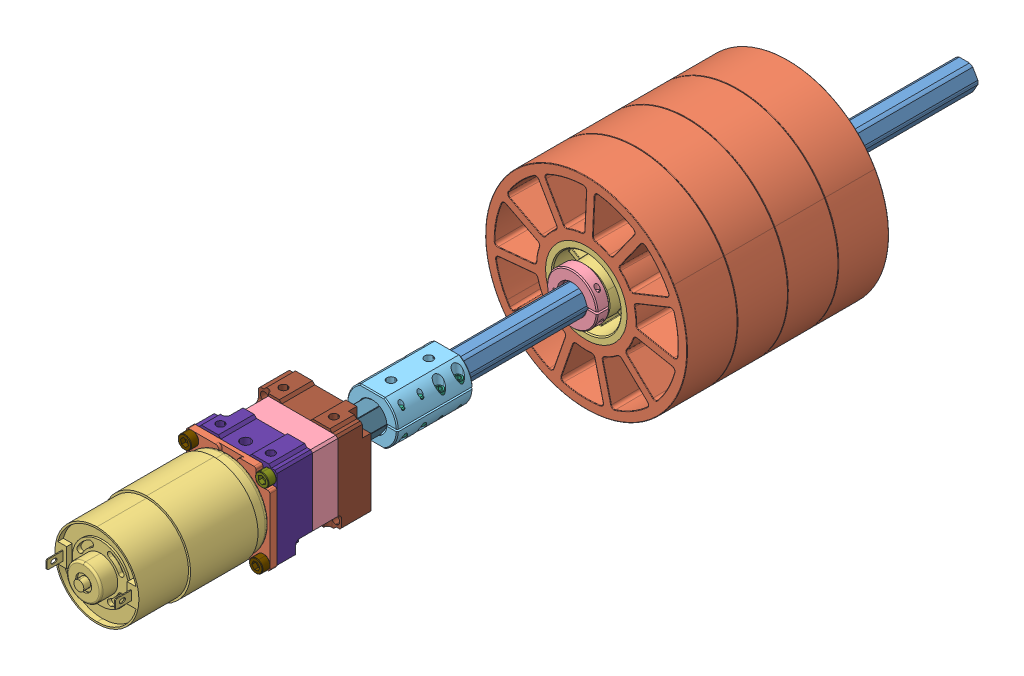
SolidWorks assembly Assem_Launch_Component(wheels,hexshaft,motor,etc.)-SP, configuration Default. Lengths in mm.
Overall size (138.79 138.79 446).
59 component instances, 25 part files, 14 mates.
Components (placement in the parent):
- ThunderHex(.5 11inch)-SP-1: ThunderHex(.5 11inch)-SP [Default] at origin size (13.74 12.75 279.4)
- CompliantWheel(4inch 500)SP-1: CompliantWheel(4inch 500)SP [Default] at (15.9875 4.7838 44.7916) x (0.866025 0.5 0) z (0 0 1) size (101.6 101.6 25.4)
  - CompliantWheel(4inch 500)SP.STEP-1: CompliantWheel(4inch 500)SP.STEP [Default] at origin size (101.6 101.6 25.4)
    - 4IN Compliant Wheel FINAL Overmold.STEP-1: 4IN Compliant Wheel FINAL Overmold.STEP [Default] at (-16.2374 3.8509 18.652) size (101.6 101.6 25.4)
    - 2in Wheel Intergrated 0500 HEX Hub.STEP-1: 2in Wheel Intergrated 0500 HEX Hub.STEP [Default] at (-16.2374 3.8509 5.952) x (-1 0 0) z (0 0 -1) size (41.91 41.91 25.4)
- CompliantWheel(4inch 500)SP.STEP-1: CompliantWheel(4inch 500)SP.STEP [Default] at (15.9875 4.7838 70.1916) x (0.866025 0.5 0) z (0 0 1) size (101.6 101.6 25.4)
  - 4IN Compliant Wheel FINAL Overmold.STEP-1: 4IN Compliant Wheel FINAL Overmold.STEP [Default] at (-16.2374 3.8509 18.652) size (101.6 101.6 25.4)
  - 2in Wheel Intergrated 0500 HEX Hub.STEP-1: 2in Wheel Intergrated 0500 HEX Hub.STEP [Default] at (-16.2374 3.8509 5.952) x (-1 0 0) z (0 0 -1) size (41.91 41.91 25.4)
- CompliantWheel(4inch 500)SP.STEP-3: CompliantWheel(4inch 500)SP.STEP [Default] at (15.9875 4.7838 95.5916) x (0.866025 0.5 0) z (0 0 1) size (101.6 101.6 25.4)
  - 4IN Compliant Wheel FINAL Overmold.STEP-1: 4IN Compliant Wheel FINAL Overmold.STEP [Default] at (-16.2374 3.8509 18.652) size (101.6 101.6 25.4)
  - 2in Wheel Intergrated 0500 HEX Hub.STEP-1: 2in Wheel Intergrated 0500 HEX Hub.STEP [Default] at (-16.2374 3.8509 5.952) x (-1 0 0) z (0 0 -1) size (41.91 41.91 25.4)
- CompliantWheel(4inch 500)SP.STEP-4: CompliantWheel(4inch 500)SP.STEP [Default] at (15.9875 4.7838 120.9916) x (0.866025 0.5 0) z (0 0 1) size (101.6 101.6 25.4)
  - 4IN Compliant Wheel FINAL Overmold.STEP-1: 4IN Compliant Wheel FINAL Overmold.STEP [Default] at (-16.2374 3.8509 18.652) size (101.6 101.6 25.4)
  - 2in Wheel Intergrated 0500 HEX Hub.STEP-1: 2in Wheel Intergrated 0500 HEX Hub.STEP [Default] at (-16.2374 3.8509 5.952) x (-1 0 0) z (0 0 -1) size (41.91 41.91 25.4)
- ClampingShaftCollar(.5 in)SP-1: ClampingShaftCollar(.5 in)SP [Default] at (0 -0.2032 34.8687) size (25.39 25.4 6.35)
- ClampingShaftCollar(.5 in)SP-2: ClampingShaftCollar(.5 in)SP [Default] at (-0.8969 -0.0987 142.8187) size (25.39 25.4 6.35)
- Hex_Shaft_Coupler(.5)-SP-1: Hex_Shaft_Coupler(.5)-SP [Default] at (0.04 0 228.4754) size (25.76 22.32 38.1)
  - Hex_Shaft_Coupler(.5)-SP.STEP-1: Hex_Shaft_Coupler(.5)-SP.STEP [Default] at origin size (25.76 22.32 38.1)
    - 217-4008-001 Rev1.STEP-1: 217-4008-001 Rev1.STEP [Default] at origin size (25.38 10.66 38.1)
    - 217-4008-001 Rev1.STEP-2: 217-4008-001 Rev1.STEP [Default] x (1 0 0) z (0 0 -1) size (25.38 10.66 38.1)
    - 217-4008-002 Rev1_91251A108.STEP-1: 217-4008-002 Rev1_91251A108.STEP [Default] at (9.7928 7.025 4.7625) x (0.994016 0 -0.109231) z (0 1 0) size (4.65 4.65 12.38)
    - 217-4008-002 Rev1_91251A108.STEP-2: 217-4008-002 Rev1_91251A108.STEP [Default] at (9.7928 7.025 14.2875) x (-0.765668 0 -0.643235) z (0 1 0) size (4.65 4.65 12.38)
    - 217-4008-002 Rev1_91251A108.STEP-3: 217-4008-002 Rev1_91251A108.STEP [Default] at (-9.7928 7.025 14.2875) x (-0.114094 0 0.99347) z (0 1 0) size (4.65 4.65 12.38)
    - 217-4008-002 Rev1_91251A108.STEP-4: 217-4008-002 Rev1_91251A108.STEP [Default] at (-9.7928 7.025 4.7625) x (0.20346 0 0.979083) z (0 1 0) size (4.65 4.65 12.38)
    - 217-4008-002 Rev1_91251A108.STEP-5: 217-4008-002 Rev1_91251A108.STEP [Default] at (-9.7928 -7.025 -4.7625) x (0.20346 0 -0.979083) z (0 -1 0) size (4.65 4.65 12.38)
    - 217-4008-002 Rev1_91251A108.STEP-6: 217-4008-002 Rev1_91251A108.STEP [Default] at (-9.7928 -7.025 -14.2875) x (-0.114094 0 -0.99347) z (0 -1 0) size (4.65 4.65 12.38)
    - 217-4008-002 Rev1_91251A108.STEP-7: 217-4008-002 Rev1_91251A108.STEP [Default] at (9.7928 -7.025 -14.2875) x (-0.765668 0 0.643235) z (0 -1 0) size (4.65 4.65 12.38)
    - 217-4008-002 Rev1_91251A108.STEP-8: 217-4008-002 Rev1_91251A108.STEP [Default] at (9.7928 -7.025 -4.7625) x (0.994016 0 0.109231) z (0 -1 0) size (4.65 4.65 12.38)
- VersaPlanetaryv2_Single_Stage_10_1_with_775_Series (General_GearBox_Shell)-SP-1: VersaPlanetaryv2_Single_Stage_10_1_with_775_Series (General_GearBox_Shell)-SP [Default] at (0.0053 -22.165 285.8002) x (0 0 -1) z (1 0 0) size (166.6 51.28 52.65)
  - VersaPlanetary_v2_Single_Stage_10_1_with_775_Series (General_GearBox_Shell)-SP.STEP-1: VersaPlanetary_v2_Single_Stage_10_1_with_775_Series (General_GearBox_Shell)-SP.STEP [Default] at origin size (166.6 51.28 52.65)
    - 217-2820 Rev1_Public.STEP-1: 217-2820 Rev1_Public.STEP [Default] at (-4.6546 22.225 0) x (0 -0.456494 0.889726) z (-1 0 0) size (39.22 38.88 17.4)
      - 217-2625-100.STEP-1: 217-2625-100.STEP [Default] at origin size (39.22 38.88 12.7)
        - 217-2625-008 Rev1.STEP-1: 217-2625-008 Rev1.STEP [Default] at origin size (34.7 34.7 4.7)
        - 217-2625-010 Rev1.STEP-1: 217-2625-010 Rev1.STEP [Default] at (0 10.193 3.65) x (0.999813 0.019336 0) z (0 0 1) size (4 4 12)
        - 217-2625-010 Rev1.STEP-2: 217-2625-010 Rev1.STEP [Default] at (8.691 -5.3258 3.65) size (4 4 12)
        - 217-2625-010 Rev1.STEP-3: 217-2625-010 Rev1.STEP [Default] at (-8.691 -5.3258 3.65) size (4 4 12)
        - 217-2625-005 Rev1_Planet_Revolving_Follower01.STEP-1: 217-2625-005 Rev1_Planet_Revolving_Follower01.STEP [Default] at (8.691 -5.3258 6.35) x (0.932816 0.360354 0) z (0 0 1) size (16.89 16.89 8)
        - 217-2625-005 Rev1_Planet_Revolving_Follower01.STEP-2: 217-2625-005 Rev1_Planet_Revolving_Follower01.STEP [Default] at (-8.691 -5.3258 6.35) x (-0.932788 -0.360426 0) z (0 0 1) size (16.89 16.89 8)
        - 217-2625-005 Rev1_Planet_Revolving_Follower01.STEP-3: 217-2625-005 Rev1_Planet_Revolving_Follower01.STEP [Default] at (0 10.193 6.35) x (0.893583 0.448898 0) z (0 0 1) size (16.89 16.89 8)
      - 217-2625-007 Rev1_Public.STEP-1: 217-2625-007 Rev1_Public.STEP [Default] at (0 0 6.7) x (0.992772 0.120019 0) z (0 0 1) size (15.27 15.27 12.7)
    - 217-2625-026 Rev1.STEP-1: 217-2625-026 Rev1.STEP [Default] at (-6.5 22.225 0) x (0 -1 0) z (-1 0 0) size (44.45 42 18.12)
    - 217-2742-001 Rev4.STEP-1: 217-2742-001 Rev4.STEP [Default] at (0.2002 22.225 0) x (1 0 0) z (0 -0.092627 0.995701) size (7 28 28)
    - 217-2742-001 Rev4.STEP-2: 217-2742-001 Rev4.STEP [Default] at (8.2002 22.225 0) size (7 28 28)
    - 217-2625-017 Rev1_9714K61.STEP-1: 217-2625-017 Rev1_9714K61.STEP [Default] at (7.42 22.3002 -0.342) x (0 0.56703 0.823697) z (0 -0.823697 0.56703) size (28.51 4.98 27.43)
    - 217-2625-003 Rev1.STEP-1: 217-2625-003 Rev1.STEP [Default] at (7.4478 22.225 0) x (0 -1 0) z (1 0 0) size (17 17 64.11)
    - 217-2625-018 Rev1_98541A410.STEP-1: 217-2625-018 Rev1_98541A410.STEP [Default] at (-0.7046 22.225 0) x (1 0 0) z (0 -0.017452 0.999848) size (1 19.6 17.4)
    - 832-1750-Ring-Gear-Screw_SSA0832-0500ZC.STEP-1: 832-1750-Ring-Gear-Screw_SSA0832-0500ZC.STEP [Default] at (-30.7 4.725 -17.5) x (0 0.997447 0.071411) z (0 -0.071411 0.997447) size (6.73 48.51 6.73)
    - 832-1750-Ring-Gear-Screw_SSA0832-0500ZC.STEP-2: 832-1750-Ring-Gear-Screw_SSA0832-0500ZC.STEP [Default] at (-30.7 39.725 17.5) x (0 0.005929 0.999982) z (0 -0.999982 0.005929) size (6.73 48.51 6.73)
    - 217-2625-025 Rev1.STEP-1: 217-2625-025 Rev1.STEP [Default] at (-23.2 22.225 0) x (0 -1 0) z (-1 0 0) size (44.45 42 18)
    - 217-4649-002 Rev1_SSA0832-0500ZC.STEP-1: 217-4649-002 Rev1_SSA0832-0500ZC.STEP [Default] at (-34.2 4.2645 17.9605) x (0 0.33842 -0.940995) z (0 0.940995 0.33842) size (6.73 16.76 6.73)
    - 217-4649-002 Rev1_SSA0832-0500ZC.STEP-2: 217-4649-002 Rev1_SSA0832-0500ZC.STEP [Default] at (-34.2 40.1855 -17.9605) x (0 -0.308932 -0.951084) z (0 0.951084 -0.308932) size (6.73 16.76 6.73)
    - 217-4649-006 Rev1_SSA0004-008BA.STEP-1: 217-4649-006 Rev1_SSA0004-008BA.STEP [Default] at (-30.7 22.225 14.5) x (0 0.5 -0.866025) z (0 -0.866025 -0.5) size (7 14 7)
    - 217-4649-006 Rev1_SSA0004-008BA.STEP-2: 217-4649-006 Rev1_SSA0004-008BA.STEP [Default] at (-30.7 22.225 -14.5) x (0 -1 0) z (0 0 1) size (7 14 7)
    - 217-2822-002 Rev4.STEP-1: 217-2822-002 Rev4.STEP [Default] at (-32.45 22.225 0) x (0 -1 0) z (-1 0 0) size (42 42 5.3)
    - 217-4347-000 Rev1.STEP-1: 217-4347-000 Rev1.STEP [Default] at (-34.2 22.225 0) x (-1 0 0) z (0 1 0) size (88 44.3 44.3)
    - 217-2816-001 Rev1.STEP-1: 217-2816-001 Rev1.STEP [Default] at (-6.35 22.225 0) x (0 -1 0) z (1 0 0) size (42 42 14.51)
    - 217-4649-001 Rev1.STEP-1: 217-4649-001 Rev1.STEP [Default] at (-20.554 22.225 0) x (0 -1 0) z (1 0 0) size (18 18 13)
    - 217-4649-007 Rev1_94105A824.STEP-1: 217-4649-007 Rev1_94105A824.STEP [Default] at (-26.029 22.225 -6.7835) x (-0.996104 -0.088191 0) z (0 0 -1) size (4.83 4.83 4.77)
    - 217-2625-013 Rev2.STEP-1: 217-2625-013 Rev2.STEP [Default] at (-25.2898 22.225 0) x (0 0 1) z (-1 0 0) size (8.01 7.94 7.5)
Mates (geometry in assembly coordinates):
- Coincident1: coincident: plane of ThunderHex(.5 11inch)-SP-1 through (-3.6808 6.3754 228.6) normal (-0.866025 0.5 0); plane of CompliantWheel(4inch 500)SP-1/CompliantWheel(4inch 500)SP.STEP-1/2in Wheel Intergrated 0500 HEX Hub.STEP-1 through (-3.6808 6.3754 38.0437) normal (0.866025 -0.5 0)
- Coincident2: coincident: plane of ThunderHex(.5 11inch)-SP-1 through (3.6808 6.3754 228.6) normal (0 1 0); plane of CompliantWheel(4inch 500)SP-1/CompliantWheel(4inch 500)SP.STEP-1/2in Wheel Intergrated 0500 HEX Hub.STEP-1 through (3.6808 6.3754 38.0437) normal (0 -1 0)
- Coincident3: coincident: circle of CompliantWheel(4inch 500)SP-1/CompliantWheel(4inch 500)SP.STEP-1/2in Wheel Intergrated 0500 HEX Hub.STEP-1; plane of CompliantWheel(4inch 500)SP.STEP-1/2in Wheel Intergrated 0500 HEX Hub.STEP-1 through (-1.27 2.1997 63.4437) normal (0 0 -1)
- Coincident4: coincident: circle of CompliantWheel(4inch 500)SP.STEP-1/4IN Compliant Wheel FINAL Overmold.STEP-1; plane of CompliantWheel(4inch 500)SP.STEP-3/2in Wheel Intergrated 0500 HEX Hub.STEP-1 through (-1.27 2.1997 88.8437) normal (0 0 -1)
- Coincident5: coincident: circle of CompliantWheel(4inch 500)SP.STEP-3/2in Wheel Intergrated 0500 HEX Hub.STEP-1; plane of CompliantWheel(4inch 500)SP.STEP-4/2in Wheel Intergrated 0500 HEX Hub.STEP-1 through (-1.27 2.1997 114.2437) normal (0 0 -1)
- Coincident7: coincident: plane of CompliantWheel(4inch 500)SP-1/CompliantWheel(4inch 500)SP.STEP-1/2in Wheel Intergrated 0500 HEX Hub.STEP-1 through (-1.27 2.1997 38.0437) normal (0 0 -1); plane of ClampingShaftCollar(.5 in)SP-1 through (0 -0.2032 38.0437) normal (0 0 1)
- Coincident8: coincident: plane of ThunderHex(.5 11inch)-SP-1 through (-3.6808 6.3754 228.6) normal (-0.866025 0.5 0); plane of ClampingShaftCollar(.5 in)SP-1 through (-3.7395 6.2738 31.6937) normal (0.866025 -0.5 0)
- Coincident9: coincident: plane of ThunderHex(.5 11inch)-SP-1 through (7.3617 0 228.6) normal (0.866025 0.5 0); plane of ClampingShaftCollar(.5 in)SP-1 through (7.479 -0.2032 31.6937) normal (-0.866025 -0.5 0)
- Coincident13: coincident: plane of CompliantWheel(4inch 500)SP.STEP-4/2in Wheel Intergrated 0500 HEX Hub.STEP-1 through (-1.27 2.1997 139.6437) normal (0 0 1); plane of ClampingShaftCollar(.5 in)SP-2 through (-0.8969 -0.0987 139.6437) normal (0 0 -1)
- Coincident16: coincident: plane of ThunderHex(.5 11inch)-SP-1 through (0 0 228.6) normal (0 0 1); plane of VersaPlanetaryv2_Single_Stage_10_1_with_775_Series (General_GearBox_Shell)-SP-1/VersaPlanetary_v2_Single_Stage_10_1_with_775_Series (General_GearBox_Shell)-SP.STEP-1/217-2625-003 Rev1.STEP-1 through (3.6715 6.41 228.6) normal (0 0 -1)
- Coincident17: coincident: plane of ThunderHex(.5 11inch)-SP-1 through (-7.3617 0 228.6) normal (-0.866025 -0.5 0); plane of Hex_Shaft_Coupler(.5)-SP-1/Hex_Shaft_Coupler(.5)-SP.STEP-1/217-4008-001 Rev1.STEP-2 through (-3.6609 -6.41 247.5254) normal (0.866025 0.5 0)
- Coincident18: coincident: plane of ThunderHex(.5 11inch)-SP-1 through (-3.6808 6.3754 228.6) normal (-0.866025 0.5 0); plane of Hex_Shaft_Coupler(.5)-SP-1/Hex_Shaft_Coupler(.5)-SP.STEP-1/217-4008-001 Rev1.STEP-1 through (-3.6609 6.41 209.4254) normal (0.866025 -0.5 0)
- Coincident21: coincident: plane of Hex_Shaft_Coupler(.5)-SP-1/Hex_Shaft_Coupler(.5)-SP.STEP-1/217-4008-001 Rev1.STEP-1 through (-3.6609 6.41 209.4254) normal (0.866025 -0.5 0); plane of VersaPlanetaryv2_Single_Stage_10_1_with_775_Series (General_GearBox_Shell)-SP-1/VersaPlanetary_v2_Single_Stage_10_1_with_775_Series (General_GearBox_Shell)-SP.STEP-1/217-2625-003 Rev1.STEP-1 through (-7.327 0.06 228.6) normal (-0.866025 0.5 0)
- Coincident22: coincident: plane of Hex_Shaft_Coupler(.5)-SP-1/Hex_Shaft_Coupler(.5)-SP.STEP-1/217-4008-001 Rev1.STEP-1 through (3.7408 6.41 209.4254) normal (0 -1 0); plane of VersaPlanetaryv2_Single_Stage_10_1_with_775_Series (General_GearBox_Shell)-SP-1/VersaPlanetary_v2_Single_Stage_10_1_with_775_Series (General_GearBox_Shell)-SP.STEP-1/217-2625-003 Rev1.STEP-1 through (-3.6609 6.41 228.6) normal (0 1 0)
